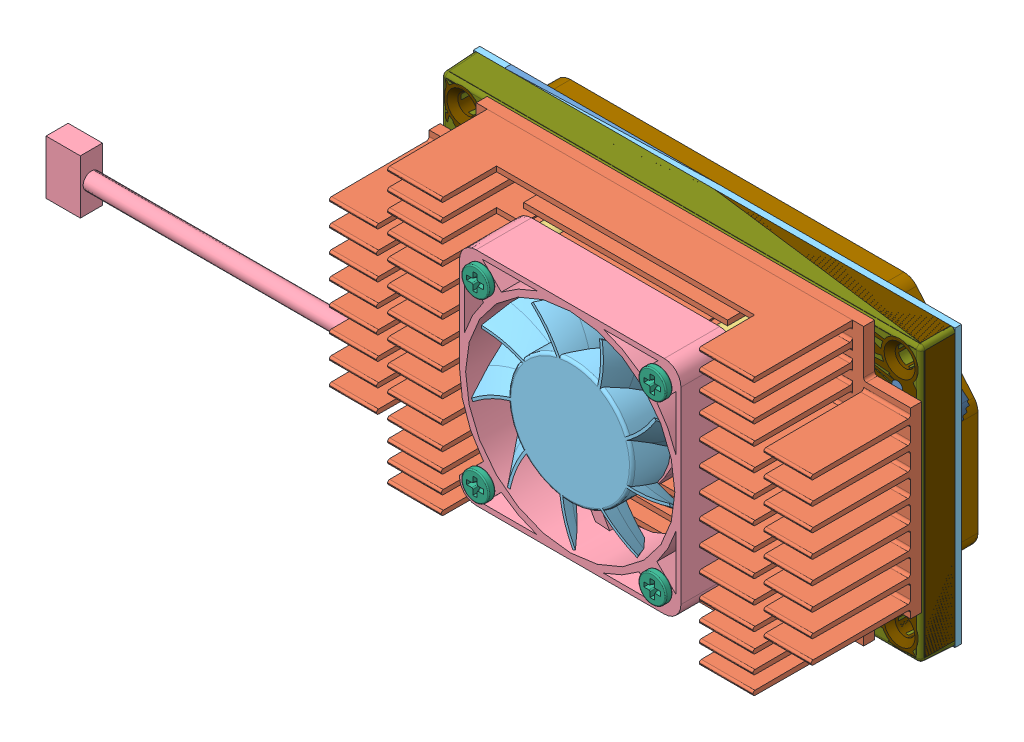
SolidWorks assembly JETSON-NEW_ASM, configuration Default. Lengths in mm. (continued)
Components (placement in the parent): (continued)
- 244-82180-1000-A01-07-31-15_ASM-1: 244-82180-1000-A01-07-31-15_ASM [Default] at origin size (87 50 8.3) (continued)
  - 195-2469-000_1-1: 195-2469-000_1 [Default] at (57.403 38.754 0) x (0 -1 0) z (0 0 -1) size (0.69 0.32 0.31)
  - 195-1636-000_1-61: 195-1636-000_1 [Default] at (57.19 37.076 0) x (-1 0 0) z (0 0 -1) size (0.69 0.32 0.31)
  - 195-1636-000_1-62: 195-1636-000_1 [Default] at (56.433 18.954 0) x (0 -1 0) z (0 0 -1) size (0.69 0.32 0.31)
  - 195-1636-000_1-63: 195-1636-000_1 [Default] at (56.153 17.514 0) x (1 0 0) z (0 0 -1) size (0.69 0.32 0.31)
  - 195-2006-000_1-13: 195-2006-000_1 [Default] at (56.153 18.064 0) x (1 0 0) z (0 0 -1) size (0.69 0.32 0.31)
  - 195-1636-000_1-64: 195-1636-000_1 [Default] at (56.153 16.294 0) x (-1 0 0) z (0 0 -1) size (0.69 0.32 0.31)
  - 195-2005-000_1-20: 195-2005-000_1 [Default] at (55.41 37.136 0) x (-1 0 0) z (0 0 -1) size (0.69 0.32 0.31)
  - 195-2005-000_1-21: 195-2005-000_1 [Default] at (54.515 37.047 0) x (1 0 0) z (0 0 -1) size (0.69 0.32 0.31)
  - 195-2004-000_1-2: 195-2004-000_1 [Default] at (54.515 36.527 0) x (1 0 0) z (0 0 -1) size (0.69 0.32 0.31)
  - 195-2004-000_1-3: 195-2004-000_1 [Default] at (54.515 36.007 0) x (1 0 0) z (0 0 -1) size (0.69 0.32 0.31)
  - 195-1636-000_1-65: 195-1636-000_1 [Default] at (56.3 37.076 0) x (1 0 0) z (0 0 -1) size (0.69 0.32 0.31)
  - 195-1636-000_1-66: 195-1636-000_1 [Default] at (69.95 41.15 0) x (-1 0 0) z (0 0 -1) size (0.69 0.32 0.31)
  - 039-0165-000_1-112: 039-0165-000_1 [Default] at (55.853 18.829 0) x (0 1 0) z (0 0 -1) size (0.69 0.32 0.34)
  - 195-2005-000_1-22: 195-2005-000_1 [Default] at (55.328 18.829 0) x (0 -1 0) z (0 0 -1) size (0.69 0.32 0.31)
  - 195-2173-000_1-1: 195-2173-000_1 [Default] at (55.063 17.794 0) x (-1 0 0) z (0 0 -1) size (0.69 0.32 0.31)
  - 195-2173-000_1-2: 195-2173-000_1 [Default] at (55.083 17.234 0) x (1 0 0) z (0 0 -1) size (0.69 0.32 0.31)
  - 039-0165-000_1-113: 039-0165-000_1 [Default] at (60.953 36.318 0) x (0 -1 0) z (0 0 -1) size (0.69 0.32 0.34)
  - 039-0165-000_1-114: 039-0165-000_1 [Default] at (59.253 34.954 0) x (1 0 0) z (0 0 -1) size (0.69 0.32 0.34)
  - 195-1636-000_1-67: 195-1636-000_1 [Default] at (59.32 33.596 0) x (0 1 0) z (0 0 -1) size (0.69 0.32 0.31)
  - 195-1636-000_1-68: 195-1636-000_1 [Default] at (59.85 33.596 0) x (0 1 0) z (0 0 -1) size (0.69 0.32 0.31)
  - 195-1636-000_1-69: 195-1636-000_1 [Default] at (61.26 31.736 0) x (-1 0 0) z (0 0 -1) size (0.69 0.32 0.31)
  - 195-1636-000_1-70: 195-1636-000_1 [Default] at (61.26 31.206 0) x (-1 0 0) z (0 0 -1) size (0.69 0.32 0.31)
  - 195-1636-000_1-71: 195-1636-000_1 [Default] at (58.65 38.25 0) x (0 1 0) z (0 0 -1) size (0.69 0.32 0.31)
  - 195-1636-000_1-72: 195-1636-000_1 [Default] at (58.103 37.754 0) x (0 -1 0) z (0 0 -1) size (0.69 0.32 0.31)
  - 039-0165-000_1-115: 039-0165-000_1 [Default] at (57.953 38.754 0) x (0 -1 0) z (0 0 -1) size (0.69 0.32 0.34)
  - 039-0165-000_1-116: 039-0165-000_1 [Default] at (58.08 36.986 0) x (1 0 0) z (0 0 -1) size (0.69 0.32 0.34)
  - 039-0165-000_1-117: 039-0165-000_1 [Default] at (58.06 36.446 0) x (1 0 0) z (0 0 -1) size (0.69 0.32 0.34)
  - 195-2005-000_1-23: 195-2005-000_1 [Default] at (61.853 39.434 0) x (1 0 0) z (0 0 -1) size (0.69 0.32 0.31)
  - 195-1636-000_1-73: 195-1636-000_1 [Default] at (62.063 38.899 0) x (1 0 0) z (0 0 -1) size (0.69 0.32 0.31)
  - 195-2117-000_1-9: 195-2117-000_1 [Default] at (62.2 37.35 0) x (1 0 0) z (0 0 -1) size (0.69 0.32 0.31)
  - 195-2350-000_1-1: 195-2350-000_1 [Default] at (62.2 35.7 0) x (1 0 0) z (0 0 -1) size (0.69 0.32 0.31)
  - 195-1636-000_1-74: 195-1636-000_1 [Default] at (61.31 33.856 0) x (1 0 0) z (0 0 -1) size (0.69 0.32 0.31)
  - 195-1636-000_1-75: 195-1636-000_1 [Default] at (61.31 33.326 0) x (1 0 0) z (0 0 -1) size (0.69 0.32 0.31)
  - 035-0122-000_1-15: 035-0122-000_1 [Default] at (61.585 32.427 1.164) x (-1 0 0) z (0 0 1) size (0.69 0.32 0.34)
  - 195-1636-000_1-76: 195-1636-000_1 [Default] at (61.31 32.796 0) x (1 0 0) z (0 0 -1) size (0.69 0.32 0.31)
  - 195-2171-000_1-3: 195-2171-000_1 [Default] at (61.98 31.446 0) x (0 1 0) z (0 0 -1) size (0.69 0.32 0.31)
  - 195-2171-000_1-4: 195-2171-000_1 [Default] at (62.7 31.736 0) x (-1 0 0) z (0 0 -1) size (0.69 0.32 0.31)
  - 195-2171-000_1-5: 195-2171-000_1 [Default] at (62.7 31.206 0) x (-1 0 0) z (0 0 -1) size (0.69 0.32 0.31)
  - 195-2006-000_1-14: 195-2006-000_1 [Default] at (61.35 17 0) x (-1 0 0) z (0 0 -1) size (0.69 0.32 0.31)
  - 195-2006-000_1-15: 195-2006-000_1 [Default] at (67.003 18.404 0) x (1 0 0) z (0 0 -1) size (0.69 0.32 0.31)
  - 195-1636-000_1-77: 195-1636-000_1 [Default] at (63.447 36.441 0) x (1 0 0) z (0 0 -1) size (0.69 0.32 0.31)
  - 195-2006-000_1-16: 195-2006-000_1 [Default] at (60.735 35.528 0) x (1 0 0) z (0 0 -1) size (0.69 0.32 0.31)
  - 195-2005-000_1-24: 195-2005-000_1 [Default] at (70.6 26.95 0) x (0 1 0) z (0 0 -1) size (0.69 0.32 0.31)
  - 195-1636-000_1-78: 195-1636-000_1 [Default] at (69 26.8 0) x (1 0 0) z (0 0 -1) size (0.69 0.32 0.31)
  - 195-2005-000_1-25: 195-2005-000_1 [Default] at (68.818 25.999 0) x (0 -1 0) z (0 0 -1) size (0.69 0.32 0.31)
  - 195-2173-000_1-3: 195-2173-000_1 [Default] at (68.073 25.764 0) x (-1 0 0) z (0 0 -1) size (0.69 0.32 0.31)
  - 195-1636-000_1-79: 195-1636-000_1 [Default] at (68.053 24.804 0) x (0 1 0) z (0 0 -1) size (0.69 0.32 0.31)
  - 195-2006-000_1-17: 195-2006-000_1 [Default] at (69.153 24.484 0) x (0 -1 0) z (0 0 -1) size (0.69 0.32 0.31)
  - 195-1636-000_1-80: 195-1636-000_1 [Default] at (68.913 25.224 0) x (1 0 0) z (0 0 -1) size (0.69 0.32 0.31)
  - 195-1636-000_1-81: 195-1636-000_1 [Default] at (68.603 24.484 0) x (0 -1 0) z (0 0 -1) size (0.69 0.32 0.31)
  - 035-0135-000_1-3: 035-0135-000_1 [Default] at (69.153 19.404 0) x (0 -1 0) z (0 0 -1) size (0.69 0.32 0.34)
  - 195-2274-000_1-1: 195-2274-000_1 [Default] at (68.553 19.404 0) x (0 -1 0) z (0 0 -1) size (0.69 0.32 0.31)
  - 039-0219-000_1-1: 039-0219-000_1 [Default] at (67.753 18.304 0) x (0 -1 0) z (0 0 -1) size (0.69 0.32 0.34)
  - 035-0135-000_1-4: 035-0135-000_1 [Default] at (68.653 18.604 0) x (1 0 0) z (0 0 -1) size (0.69 0.32 0.34)
  - 195-2173-000_1-4: 195-2173-000_1 [Default] at (67.133 25.764 0) x (1 0 0) z (0 0 -1) size (0.69 0.32 0.31)
  - 195-2004-000_1-4: 195-2004-000_1 [Default] at (18.25 37.45 0) x (0 1 0) z (0 0 -1) size (0.69 0.32 0.31)
  - 195-2004-000_1-5: 195-2004-000_1 [Default] at (18.8 37.45 0) x (0 1 0) z (0 0 -1) size (0.69 0.32 0.31)
  - 195-1636-000_1-82: 195-1636-000_1 [Default] at (41.75 9 1.164) x (0 -1 0) z (0 0 1) size (0.69 0.32 0.31)
  - 195-2459-000_1-1: 195-2459-000_1 [Default] at (70.675 24.972 0) x (0 1 0) z (0 0 -1) size (0.69 0.32 0.31)
  - 195-1636-000_1-83: 195-1636-000_1 [Default] at (70.053 24.254 0) x (1 0 0) z (0 0 -1) size (0.69 0.32 0.31)
  - 039-0165-000_1-118: 039-0165-000_1 [Default] at (69.903 24.854 0) x (1 0 0) z (0 0 -1) size (0.69 0.32 0.34)
  - 195-1636-000_1-84: 195-1636-000_1 [Default] at (70.753 20.604 0) x (0 -1 0) z (0 0 -1) size (0.69 0.32 0.31)
  - 035-0135-000_1-5: 035-0135-000_1 [Default] at (70.553 19.284 0) x (1 0 0) z (0 0 -1) size (0.69 0.32 0.34)
  - 195-2172-000_1-4: 195-2172-000_1 [Default] at (70.553 19.804 0) x (1 0 0) z (0 0 -1) size (0.69 0.32 0.31)
  - 035-0135-000_1-6: 035-0135-000_1 [Default] at (69.753 19.404 0) x (0 -1 0) z (0 0 -1) size (0.69 0.32 0.34)
  - 195-2172-000_1-5: 195-2172-000_1 [Default] at (70.253 18.004 0) x (1 0 0) z (0 0 -1) size (0.69 0.32 0.31)
  - 195-1636-000_1-85: 195-1636-000_1 [Default] at (70.253 18.604 0) x (1 0 0) z (0 0 -1) size (0.69 0.32 0.31)
  - 035-0135-000_1-7: 035-0135-000_1 [Default] at (71.25 18 0) x (1 0 0) z (0 0 -1) size (0.69 0.32 0.34)
  - 195-2002-000_1-6: 195-2002-000_1 [Default] at (68.9 33 0) x (0 1 0) z (0 0 -1) size (0.69 0.32 0.31)
  - 195-2002-000_1-7: 195-2002-000_1 [Default] at (73.4 30.6 0) x (1 0 0) z (0 0 -1) size (0.69 0.32 0.31)
  - 195-2319-000_1-1: 195-2319-000_1 [Default] at (70.953 23.922 0) x (-1 0 0) z (0 0 -1) size (0.69 0.32 0.31)
  - 039-0199-000_1-2: 039-0199-000_1 [Default] at (70.953 22.804 0) x (1 0 0) z (0 0 -1) size (0.69 0.32 0.36)
  - 195-2299-000_1-1: 195-2299-000_1 [Default] at (71.853 22.804 0) x (-1 0 0) z (0 0 -1) size (0.69 0.32 0.31)
  - 195-2289-000_1-1: 195-2289-000_1 [Default] at (70.953 23.404 0) x (1 0 0) z (0 0 -1) size (0.69 0.32 0.31)
  - 195-1636-000_1-86: 195-1636-000_1 [Default] at (71.853 23.404 0) x (1 0 0) z (0 0 -1) size (0.69 0.32 0.31)
  - 032-0335-000_1-1: 032-0335-000_1 [Default] at (71.553 20.804 0) x (-1 0 0) z (0 0 -1) size (0.69 0.32 0.34)
  - 195-2173-000_1-5: 195-2173-000_1 [Default] at (70.953 21.404 0) x (-1 0 0) z (0 0 -1) size (0.69 0.32 0.31)
  - 195-2061-000_1-1: 195-2061-000_1 [Default] at (71.853 21.404 0) x (-1 0 0) z (0 0 -1) size (0.69 0.32 0.31)
  - 195-2548-000_1-1: 195-2548-000_1 [Default] at (70.953 22.204 0) x (1 0 0) z (0 0 -1) size (0.69 0.32 0.31)
  - 039-0165-000_1-119: 039-0165-000_1 [Default] at (71.853 22.204 0) x (1 0 0) z (0 0 -1) size (0.69 0.32 0.34)
  - 195-1636-000_1-87: 195-1636-000_1 [Default] at (72.5 19.9 0) x (1 0 0) z (0 0 -1) size (0.69 0.32 0.31)
  - 195-2003-000_1-1: 195-2003-000_1 [Default] at (71.25 18.6 0) x (1 0 0) z (0 0 -1) size (0.69 0.32 0.31)
  - 036-0107-000_1-1: 036-0107-000_1 [Default] at (71.553 19.304 0) x (1 0 0) z (0 0 -1) size (0.69 0.32 0.31)
  - 195-1636-000_1-88: 195-1636-000_1 [Default] at (71.553 19.904 0) x (1 0 0) z (0 0 -1) size (0.69 0.32 0.31)
  - 195-1636-000_1-89: 195-1636-000_1 [Default] at (72.5 19.3 0) x (1 0 0) z (0 0 -1) size (0.69 0.32 0.31)
  - 195-2003-000_1-2: 195-2003-000_1 [Default] at (72.5 20.45 0) x (1 0 0) z (0 0 -1) size (0.69 0.32 0.31)
  - 195-2002-000_1-8: 195-2002-000_1 [Default] at (74.5 30.3 0) x (1 0 0) z (0 0 -1) size (0.69 0.32 0.31)
  - 195-2002-000_1-9: 195-2002-000_1 [Default] at (77.75 33.4 0) x (1 0 0) z (0 0 -1) size (0.69 0.32 0.31)
  - 195-1636-000_1-90: 195-1636-000_1 [Default] at (74.65 29.5 0) x (0 1 0) z (0 0 -1) size (0.69 0.32 0.31)
  - 195-2002-000_1-10: 195-2002-000_1 [Default] at (73.55 31.15 0) x (-1 0 0) z (0 0 -1) size (0.69 0.32 0.31)
  - 195-1636-000_1-91: 195-1636-000_1 [Default] at (74.55 37.6 0) x (0 -1 0) z (0 0 -1) size (0.69 0.32 0.31)
  - 035-0243-000_2-23: 035-0243-000_2 [Default] at (21.1 29.15 1.164) x (0 -1 0) z (0 0 1) size (0.69 0.32 0.34)
  - 035-0243-000_2-24: 035-0243-000_2 [Default] at (22.3 24.7 1.164) x (-1 0 0) z (0 0 1) size (0.69 0.32 0.34)
  - 195-2004-000_1-6: 195-2004-000_1 [Default] at (18.35 20.85 1.164) size (0.69 0.32 0.31)
  - 195-2004-000_1-7: 195-2004-000_1 [Default] at (18.35 21.4 1.164) size (0.69 0.32 0.31)
  - 195-2057-000_1-1: 195-2057-000_1 [Default] at (26.4 22.45 1.164) x (0 -1 0) z (0 0 1) size (0.69 0.32 0.31)
  - 195-2117-000_1-10: 195-2117-000_1 [Default] at (17.2 23.15 0) x (1 0 0) z (0 0 -1) size (0.69 0.32 0.31)
  - 195-2117-000_1-11: 195-2117-000_1 [Default] at (17.2 24.25 0) x (1 0 0) z (0 0 -1) size (0.69 0.32 0.31)
  - 195-2117-000_1-12: 195-2117-000_1 [Default] at (18.55 15.5 0) x (1 0 0) z (0 0 -1) size (0.69 0.32 0.31)
  - 195-2117-000_1-13: 195-2117-000_1 [Default] at (17.6 15.5 0) x (1 0 0) z (0 0 -1) size (0.69 0.32 0.31)
  - 195-2117-000_1-14: 195-2117-000_1 [Default] at (17.6 17.19 0) x (1 0 0) z (0 0 -1) size (0.69 0.32 0.31)
  - 195-1636-000_1-92: 195-1636-000_1 [Default] at (19.785 34.602 0) x (0 1 0) z (0 0 -1) size (0.69 0.32 0.31)
  - 195-1636-000_1-93: 195-1636-000_1 [Default] at (19.267 34.602 0) x (0 1 0) z (0 0 -1) size (0.69 0.32 0.31)
  - 195-1636-000_1-94: 195-1636-000_1 [Default] at (51.7 24.8 0) x (0 1 0) z (0 0 -1) size (0.69 0.32 0.31)
  - 035-0243-000_2-25: 035-0243-000_2 [Default] at (48.05 23.5 1.164) x (0 1 0) z (0 0 1) size (0.69 0.32 0.34)
  - 039-0165-000_1-120: 039-0165-000_1 [Default] at (41.543 22.374 0) x (0 -1 0) z (0 0 -1) size (0.69 0.32 0.34)
  - 039-0165-000_1-121: 039-0165-000_1 [Default] at (40.833 22.824 0) x (-1 0 0) z (0 0 -1) size (0.69 0.32 0.34)
  - 195-2007-000_1-1: 195-2007-000_1 [Default] at (18.65 12.6 0) x (0 -1 0) z (0 0 -1) size (0.69 0.32 0.31)
  - 195-1636-000_1-95: 195-1636-000_1 [Default] at (-0.85 36.75 1.164) x (-1 0 0) z (0 0 1) size (0.69 0.32 0.31)
  - 035-0243-000_2-26: 035-0243-000_2 [Default] at (-0.1 36.5 1.164) x (0 -1 0) z (0 0 1) size (0.69 0.32 0.34)
  - 035-0105-000_1-9: 035-0105-000_1 [Default] at (0.65 36.75 1.164) size (0.69 0.32 0.34)
  - 195-1636-000_1-96: 195-1636-000_1 [Default] at (-0.85 31.15 1.164) x (-1 0 0) z (0 0 1) size (0.69 0.32 0.31)
  - 035-0243-000_2-27: 035-0243-000_2 [Default] at (-0.1 30.9 1.164) x (0 -1 0) z (0 0 1) size (0.69 0.32 0.34)
  - 035-0105-000_1-10: 035-0105-000_1 [Default] at (0.65 31.15 1.164) size (0.69 0.32 0.34)
  - 035-0122-000_1-16: 035-0122-000_1 [Default] at (57.665 22.463 0) x (0 -1 0) z (0 0 -1) size (0.69 0.32 0.34)
  - 195-2566-000_1-1: 195-2566-000_1 [Default] at (31.05 10.1 1.164) x (0 -1 0) z (0 0 1) size (0.69 0.32 0.31)
  - 195-1636-000_1-97: 195-1636-000_1 [Default] at (64.54 30.986 0) x (-1 0 0) z (0 0 -1) size (0.69 0.32 0.31)
  - 195-1636-000_1-98: 195-1636-000_1 [Default] at (63.6 30.986 0) x (1 0 0) z (0 0 -1) size (0.69 0.32 0.31)
  - 195-1636-000_1-99: 195-1636-000_1 [Default] at (62.7 32.266 0) x (-1 0 0) z (0 0 -1) size (0.69 0.32 0.31)
  - 195-1636-000_1-100: 195-1636-000_1 [Default] at (61.26 32.266 0) x (-1 0 0) z (0 0 -1) size (0.69 0.32 0.31)
  - 036-0107-000_1-2: 036-0107-000_1 [Default] at (64.28 32.246 0) x (1 0 0) z (0 0 -1) size (0.69 0.32 0.31)
  - 195-2566-000_1-2: 195-2566-000_1 [Default] at (45.8 23.3 1.164) x (0 1 0) z (0 0 1) size (0.69 0.32 0.31)
  - 195-2319-000_1-2: 195-2319-000_1 [Default] at (56.55 19.856 0) x (0 -1 0) z (0 0 -1) size (0.69 0.32 0.31)
  - 195-2299-000_1-2: 195-2299-000_1 [Default] at (58.55 21.116 0) x (-1 0 0) z (0 0 -1) size (0.69 0.32 0.31)
  - 195-2289-000_1-2: 195-2289-000_1 [Default] at (57.09 19.856 0) x (0 1 0) z (0 0 -1) size (0.69 0.32 0.31)
  - 195-1636-000_1-101: 195-1636-000_1 [Default] at (58.55 21.656 0) x (1 0 0) z (0 0 -1) size (0.69 0.32 0.31)
  - 032-0335-000_1-2: 032-0335-000_1 [Default] at (58.55 20.576 0) x (-1 0 0) z (0 0 -1) size (0.69 0.32 0.34)
  - 039-0199-000_1-3: 039-0199-000_1 [Default] at (57.63 19.856 0) x (0 1 0) z (0 0 -1) size (0.69 0.32 0.36)
  - 039-0204-000_1-1: 039-0204-000_1 [Default] at (71.45 25.1 0) x (-1 0 0) z (0 0 -1) size (0.69 0.32 0.34)
  - 039-0204-000_1-2: 039-0204-000_1 [Default] at (58.17 19.856 0) x (0 1 0) z (0 0 -1) size (0.69 0.32 0.34)
  - 195-1636-000_1-102: 195-1636-000_1 [Default] at (71.453 24.573 0) x (1 0 0) z (0 0 -1) size (0.69 0.32 0.31)
  - 195-1636-000_1-103: 195-1636-000_1 [Default] at (58.74 19.856 0) x (0 -1 0) z (0 0 -1) size (0.69 0.32 0.31)
  - 101-0142-000_2-1: 101-0142-000_2 [Default] at (6.063 36.964 1.164) x (0 1 0) z (0 0 1) size (1.4 1.1 0.4)
  - 101-0142-000_2-2: 101-0142-000_2 [Default] at (5.31 31.454 1.164) x (0 1 0) z (0 0 1) size (1.4 1.1 0.4)
  - 085-0203-000_1-1: 085-0203-000_1 [Default] at (13.653 29.754 1.164) size (1.75 1.35 0.4)
  - 131-0802-000_2-1: 131-0802-000_2 [Default] at (18.469 28.798 1.164) x (0 -1 0) z (0 0 1) size (2.53 1.61 1.01)
  - 085-0180-000_1-1: 085-0180-000_1 [Default] at (23.25 23 1.164) x (-1 0 0) z (0 0 1) size (2.9 2.5 0.56)
  - 305-0057-000_1-1: 305-0057-000_1 [Default] at (41.153 40.254 0) x (1 0 0) z (0 0 -1) size (2 2.69 1.1)
  - 115-0057-000_1-1: 115-0057-000_1 [Default] at (1.1 13.65 0) x (-1 0 0) z (0 0 -1) size (2 2.88 1.1)
  - 115-1572-000_1-1: 115-1572-000_1 [Default] at (65.88 15.256 0) x (0 -1 0) z (0 0 -1) size (2 2.88 1.1)
  - 315-0217-000_1-1: 315-0217-000_1 [Default] at (41.273 36.727 0) x (1 0 0) z (0 0 -1) size (2 2.88 1.1)
  - 032-0627-000_1-1: 032-0627-000_1 [Default] at (1.38 7.93 1.164) x (-1 0 0) z (0 0 1) size (4.22 2.82 1.2)
  - 032-0627-000_1-2: 032-0627-000_1 [Default] at (68.106 40.15 1.164) x (0 -1 0) z (0 0 1) size (4.22 2.82 1.2)
  - 032-0627-000_1-3: 032-0627-000_1 [Default] at (72.09 40.46 1.164) size (4.22 2.82 1.2)
  - 032-0627-000_1-4: 032-0627-000_1 [Default] at (1.38 11.27 1.164) x (-1 0 0) z (0 0 1) size (4.22 2.82 1.2)
  - 032-0636-000_1-1: 032-0636-000_1 [Default] at (47.778 13.049 0) x (1 0 0) z (0 0 -1) size (4.22 2.82 1.5)
  - 032-0471-000_2-1: 032-0471-000_2 [Default] at (47.78 16.326 0) x (1 0 0) z (0 0 -1) size (4.22 2.82 1.2)
  - 032-0636-000_1-2: 032-0636-000_1 [Default] at (54.36 22.056 0) x (0 -1 0) z (0 0 -1) size (4.22 2.82 1.5)
  - 032-0471-000_2-2: 032-0471-000_2 [Default] at (36.91 17.143 0) x (-1 0 0) z (0 0 -1) size (4.22 2.82 1.2)
  - 032-0471-000_2-3: 032-0471-000_2 [Default] at (49.67 19.576 0) x (1 0 0) z (0 0 -1) size (4.22 2.82 1.2)
  - 130-0646-000_1-1: 130-0646-000_1 [Default] at (57.753 23.554 1.164) x (-1 0 0) z (0 0 1) size (8.4 6.6 1.8)
  - 130-0646-000_1-2: 130-0646-000_1 [Default] at (57.753 16.304 1.164) x (-1 0 0) z (0 0 1) size (8.4 6.6 1.8)
  - 130-0562-000_2-1: 130-0562-000_2 [Default] at (56.978 30.96 1.164) x (0 -1 0) z (0 0 1) size (2.8 2.25 1.22)
  - 130-0562-000_2-2: 130-0562-000_2 [Default] at (53.858 37.854 1.164) x (0 1 0) z (0 0 1) size (2.8 2.25 1.22)
  - 130-0562-000_2-3: 130-0562-000_2 [Default] at (53.848 33.894 1.164) x (0 -1 0) z (0 0 1) size (2.8 2.25 1.22)
  - 130-0562-000_2-4: 130-0562-000_2 [Default] at (59.478 30.965 1.164) x (0 -1 0) z (0 0 1) size (2.8 2.25 1.22)
  - 130-0562-000_2-5: 130-0562-000_2 [Default] at (63.578 33.764 1.164) x (0 -1 0) z (0 0 1) size (2.8 2.25 1.22)
  - 300-0252-000_1-1: 300-0252-000_1 [Default] at (63.7 17.8 1.164) x (0 -1 0) z (0 0 1) size (3.81 3.5 0.81)
  - 300-0252-000_1-2: 300-0252-000_1 [Default] at (63.7 22.25 1.164) x (0 1 0) z (0 0 1) size (3.81 3.5 0.81)
  - 300-0252-000_1-3: 300-0252-000_1 [Default] at (63.7 13.55 1.164) x (0 1 0) z (0 0 1) size (3.81 3.5 0.81)
  - 300-0252-000_1-4: 300-0252-000_1 [Default] at (63.7 26.5 1.164) x (0 -1 0) z (0 0 1) size (3.81 3.5 0.81)
  - 300-0284-000_1-1: 300-0284-000_1 [Default] at (67.9 22.7 1.164) size (3.81 3.5 0.81)
  - 300-0284-000_1-2: 300-0284-000_1 [Default] at (67.9 15.45 1.164) size (3.81 3.5 0.81)
  - 039-0208-000_1-1: 039-0208-000_1 [Default] at (4.01 9.61 1.164) x (0 1 0) z (0 0 1) size (1.2 0.5 0.55)
  - 039-0208-000_1-2: 039-0208-000_1 [Default] at (73.36 37.97 1.164) size (1.2 0.5 0.55)
  - 032-0204-000_2-1: 032-0204-000_2 [Default] at (69.95 26.3 0) x (0 1 0) z (0 0 -1) size (1.2 0.5 0.55)
  - 195-0486-000_1-1: 195-0486-000_1 [Default] at (9.75 33.6 0) x (-1 0 0) z (0 0 -1) size (1.2 0.5 0.4)
  - 195-0324-000_1-1: 195-0324-000_1 [Default] at (10.2 30.95 0) x (0 -1 0) z (0 0 -1) size (1.2 0.5 0.4)
  - 195-0235-000_1-1: 195-0235-000_1 [Default] at (9.4 32.45 0) x (0 -1 0) z (0 0 -1) size (1.2 0.5 0.4)
  - 036-0014-000_1-1: 036-0014-000_1 [Default] at (6.25 30.3 0) x (1 0 0) z (0 0 -1) size (1.2 0.5 0.6)
  - 036-0014-000_1-2: 036-0014-000_1 [Default] at (9.4 30.95 0) x (0 -1 0) z (0 0 -1) size (1.2 0.5 0.6)
  - 195-1691-000_1-1: 195-1691-000_1 [Default] at (44.62 11.876 0) x (0 1 0) z (0 0 -1) size (1.2 0.5 0.4)
  - 195-1691-000_1-2: 195-1691-000_1 [Default] at (43.89 11.876 0) x (0 1 0) z (0 0 -1) size (1.2 0.5 0.4)
  - 195-0415-000_1-1: 195-0415-000_1 [Default] at (74.79 39.5 1.164) x (0 1 0) z (0 0 1) size (1.2 0.5 0.4)
  - 035-0017-000_1-1: 035-0017-000_1 [Default] at (76.18 34.056 1.164) x (0 -1 0) z (0 0 1) size (1.2 0.5 0.6)
  - 195-0210-000_1-1: 195-0210-000_1 [Default] at (77.99 35.336 1.164) size (1.2 0.5 0.4)
  - 195-0475-000_1-1: 195-0475-000_1 [Default] at (77.98 34.596 1.164) x (-1 0 0) z (0 0 1) size (1.2 0.5 0.4)
  - 036-0141-000_1-1: 036-0141-000_1 [Default] at (76.93 34.056 1.164) x (0 -1 0) z (0 0 1) size (1.2 0.5 0.61)
  - 195-0070-000_1-1: 195-0070-000_1 [Default] at (76.53 35.156 1.164) size (1.2 0.5 0.4)
  - 035-0212-000_1-1: 035-0212-000_1 [Default] at (77.69 32.384 1.164) x (0 1 0) z (0 0 1) size (1.2 0.5 0.55)
  - 195-0005-000_1-1: 195-0005-000_1 [Default] at (76.97 32.384 1.164) x (0 1 0) z (0 0 1) size (1.2 0.5 0.4)
  - 195-0140-000_1-1: 195-0140-000_1 [Default] at (75.74 32.814 1.164) x (-1 0 0) z (0 0 1) size (1.2 0.5 0.4)
  - 195-0342-000_1-1: 195-0342-000_1 [Default] at (75.776 31.96 1.164) size (1.2 0.5 0.4)
  - 195-0405-000_1-1: 195-0405-000_1 [Default] at (2.04 14.56 1.164) x (-1 0 0) z (0 0 1) size (1.2 0.5 0.4)
  - 035-0212-000_1-2: 035-0212-000_1 [Default] at (8.776 12.06 1.164) x (0 -1 0) z (0 0 1) size (1.2 0.5 0.55)
  - 195-0487-000_1-1: 195-0487-000_1 [Default] at (0.83 14.77 1.164) x (0 1 0) z (0 0 1) size (1.2 0.5 0.4)
  - 195-0240-000_1-1: 195-0240-000_1 [Default] at (-0.384 15.76 1.164) x (0 -1 0) z (0 0 1) size (1.2 0.5 0.4)
  - 036-0141-000_1-2: 036-0141-000_1 [Default] at (9.126 10.96 1.164) x (-1 0 0) z (0 0 1) size (1.2 0.5 0.61)
  - 195-0404-000_1-1: 195-0404-000_1 [Default] at (9.526 12.06 1.164) x (0 -1 0) z (0 0 1) size (1.2 0.5 0.4)
  - 035-0212-000_1-3: 035-0212-000_1 [Default] at (10.24 9.756 1.164) x (0 -1 0) z (0 0 1) size (1.2 0.5 0.55)
  - 195-0342-000_1-2: 195-0342-000_1 [Default] at (11.404 10.18 1.164) x (-1 0 0) z (0 0 1) size (1.2 0.5 0.4)
  - 195-0005-000_1-2: 195-0005-000_1 [Default] at (9.53 9.756 1.164) x (0 -1 0) z (0 0 1) size (1.2 0.5 0.4)
  - 195-0250-000_1-1: 195-0250-000_1 [Default] at (8.664 9.78 1.164) x (0 1 0) z (0 0 1) size (1.2 0.5 0.4)
  - 195-0485-000_1-1: 195-0485-000_1 [Default] at (5.7 11.85 0) x (-1 0 0) z (0 0 -1) size (1.2 0.5 0.4)
  - 195-0485-000_1-2: 195-0485-000_1 [Default] at (5.7 12.6 0) x (-1 0 0) z (0 0 -1) size (1.2 0.5 0.4)
  - 039-0023-000_1-1: 039-0023-000_1 [Default] at (36.871 31.058 0) x (-1 0 0) z (0 0 -1) size (1.2 0.5 0.6)
  - 195-0031-000_1-1: 195-0031-000_1 [Default] at (35.801 30.61 0) x (0 1 0) z (0 0 -1) size (1.2 0.5 0.4)
  - 195-2655-000_1-1: 195-2655-000_1 [Default] at (36.871 30.308 0) x (-1 0 0) z (0 0 -1) size (1.2 0.5 0.4)
  - 195-0437-000_1-1: 195-0437-000_1 [Default] at (36.479 24.219 0) x (0 -1 0) z (0 0 -1) size (1.2 0.5 0.4)
  - 195-0292-000_1-1: 195-0292-000_1 [Default] at (35.427 24.921 0) x (-1 0 0) z (0 0 -1) size (1.2 0.5 0.4)
  - 039-0008-000_1-1: 039-0008-000_1 [Default] at (39.63 37.104 0) x (0 -1 0) z (0 0 -1) size (1.2 0.5 0.6)
  - 039-0008-000_1-2: 039-0008-000_1 [Default] at (41.103 34.754 0) x (1 0 0) z (0 0 -1) size (1.2 0.5 0.6)
  - 195-0484-000_1-1: 195-0484-000_1 [Default] at (46.963 29.024 0) x (1 0 0) z (0 0 -1) size (1.2 0.5 0.4)
  - 195-0596-000_1-1: 195-0596-000_1 [Default] at (46.963 28.214 0) x (1 0 0) z (0 0 -1) size (1.2 0.5 0.4)
  - 195-0002-000_1-1: 195-0002-000_1 [Default] at (52.188 28.414 0) x (-1 0 0) z (0 0 -1) size (1.2 0.5 0.4)
  - 036-0012-000_1-1: 036-0012-000_1 [Default] at (51.053 28.084 0) x (0 -1 0) z (0 0 -1) size (1.2 0.5 0.6)
  - 195-0486-000_1-2: 195-0486-000_1 [Default] at (69.45 10.95 1.164) size (1.2 0.5 0.4)
  - 039-0008-000_1-3: 039-0008-000_1 [Default] at (11.5 19.1 0) x (0 -1 0) z (0 0 -1) size (1.2 0.5 0.6)
  - 195-2655-000_1-2: 195-2655-000_1 [Default] at (19.934 31.265 0) x (0 -1 0) z (0 0 -1) size (1.2 0.5 0.4)
  - 039-0008-000_1-4: 039-0008-000_1 [Default] at (21.486 32.341 0) x (-1 0 0) z (0 0 -1) size (1.2 0.5 0.6)
  - 195-2655-000_1-3: 195-2655-000_1 [Default] at (20.641 31.27 0) x (0 -1 0) z (0 0 -1) size (1.2 0.5 0.4)
  - 039-0136-000_1-1: 039-0136-000_1 [Default] at (10.606 31.182 1.164) x (-0.707107 -0.707107 0) z (0 0 1) size (1.2 0.5 0.61)
  - 039-0136-000_1-2: 039-0136-000_1 [Default] at (12.104 29.849 1.164) x (0 1 0) z (0 0 1) size (1.2 0.5 0.61)
  - 039-0136-000_1-3: 039-0136-000_1 [Default] at (11.729 28.799 1.164) x (-1 0 0) z (0 0 1) size (1.2 0.5 0.61)
  - 039-0136-000_1-4: 039-0136-000_1 [Default] at (14.693 27.88 1.164) x (-1 0 0) z (0 0 1) size (1.2 0.5 0.61)
  - 039-0136-000_1-5: 039-0136-000_1 [Default] at (12.197 36.147 1.164) x (-1 0 0) z (0 0 1) size (1.2 0.5 0.61)
  - 039-0008-000_1-5: 039-0008-000_1 [Default] at (13.012 34.245 0) x (0 1 0) z (0 0 -1) size (1.2 0.5 0.6)
  - 195-2655-000_1-4: 195-2655-000_1 [Default] at (13.563 33.192 0) x (1 0 0) z (0 0 -1) size (1.2 0.5 0.4)
  - 039-0136-000_1-6: 039-0136-000_1 [Default] at (13.208 27.925 1.164) x (-1 0 0) z (0 0 1) size (1.2 0.5 0.61)
  - 195-2655-000_1-5: 195-2655-000_1 [Default] at (18.836 32.716 0) x (0 -1 0) z (0 0 -1) size (1.2 0.5 0.4)
  - 032-0153-000_2-1: 032-0153-000_2 [Default] at (17.436 32.716 0) x (0 1 0) z (0 0 -1) size (1.2 0.5 0.6)
  - 039-0008-000_1-6: 039-0008-000_1 [Default] at (14.75 39.45 0) x (-1 0 0) z (0 0 -1) size (1.2 0.5 0.6)
  - 195-2655-000_1-6: 195-2655-000_1 [Default] at (15.15 38.25 0) x (0 1 0) z (0 0 -1) size (1.2 0.5 0.4)
  - 039-0008-000_1-7: 039-0008-000_1 [Default] at (15.15 42.05 0) x (0 1 0) z (0 0 -1) size (1.2 0.5 0.6)
  - 039-0136-000_1-7: 039-0136-000_1 [Default] at (16.088 35.815 0) x (0 1 0) z (0 0 -1) size (1.2 0.5 0.61)
  - 039-0136-000_1-8: 039-0136-000_1 [Default] at (16.036 33.333 0) x (0 1 0) z (0 0 -1) size (1.2 0.5 0.61)
  - 039-0008-000_1-8: 039-0008-000_1 [Default] at (17.786 33.809 0) x (1 0 0) z (0 0 -1) size (1.2 0.5 0.6)
  - 039-0011-000_1-1: 039-0011-000_1 [Default] at (16.736 32.933 0) x (0 1 0) z (0 0 -1) size (1.2 0.5 0.6)
  - 039-0136-000_1-9: 039-0136-000_1 [Default] at (15.842 29.849 1.164) x (0 -1 0) z (0 0 1) size (1.2 0.5 0.61)
  - 032-0153-000_2-2: 032-0153-000_2 [Default] at (17.068 29.641 1.164) x (0 -1 0) z (0 0 1) size (1.2 0.5 0.6)
  - 195-2655-000_1-7: 195-2655-000_1 [Default] at (27.6 19.65 0) x (0 -1 0) z (0 0 -1) size (1.2 0.5 0.4)
  - 039-0008-000_1-9: 039-0008-000_1 [Default] at (26.268 14.214 0) x (0 1 0) z (0 0 -1) size (1.2 0.5 0.6)
  - 195-2655-000_1-8: 195-2655-000_1 [Default] at (24.438 17.784 0) x (1 0 0) z (0 0 -1) size (1.2 0.5 0.4)
  - 039-0008-000_1-10: 039-0008-000_1 [Default] at (25.473 16.544 0) x (0 -1 0) z (0 0 -1) size (1.2 0.5 0.6)
  - 039-0008-000_1-11: 039-0008-000_1 [Default] at (25.032 13.913 0) x (1 0 0) z (0 0 -1) size (1.2 0.5 0.6)
  - 039-0008-000_1-12: 039-0008-000_1 [Default] at (23.442 16.554 0) x (0 -1 0) z (0 0 -1) size (1.2 0.5 0.6)
  - 039-0008-000_1-13: 039-0008-000_1 [Default] at (33.563 14.704 0) x (0 1 0) z (0 0 -1) size (1.2 0.5 0.6)
  - 039-0008-000_1-14: 039-0008-000_1 [Default] at (39.241 18.025 0) x (1 0 0) z (0 0 -1) size (1.2 0.5 0.6)
  - 039-0008-000_1-15: 039-0008-000_1 [Default] at (37.923 13.224 0) x (0 -1 0) z (0 0 -1) size (1.2 0.5 0.6)
  - 039-0008-000_1-16: 039-0008-000_1 [Default] at (36.533 21.324 0) x (0 -1 0) z (0 0 -1) size (1.2 0.5 0.6)
  - 039-0008-000_1-17: 039-0008-000_1 [Default] at (36.883 19.644 0) x (0 -1 0) z (0 0 -1) size (1.2 0.5 0.6)
  - 039-0008-000_1-18: 039-0008-000_1 [Default] at (36.423 14.689 0) x (0 -1 0) z (0 0 -1) size (1.2 0.5 0.6)
  - 039-0008-000_1-19: 039-0008-000_1 [Default] at (34.543 20.894 0) x (-1 0 0) z (0 0 -1) size (1.2 0.5 0.6)
  - 039-0008-000_1-20: 039-0008-000_1 [Default] at (43.6 19.15 0) x (0 1 0) z (0 0 -1) size (1.2 0.5 0.6)
  - 039-0008-000_1-21: 039-0008-000_1 [Default] at (34.282 15.951 0) x (0 1 0) z (0 0 -1) size (1.2 0.5 0.6)
  - 039-0008-000_1-22: 039-0008-000_1 [Default] at (39.653 19.654 0) x (0 -1 0) z (0 0 -1) size (1.2 0.5 0.6)
  - 039-0008-000_1-23: 039-0008-000_1 [Default] at (40.423 13.214 0) x (0 -1 0) z (0 0 -1) size (1.2 0.5 0.6)
  - 195-2655-000_1-9: 195-2655-000_1 [Default] at (39.163 11.574 0) x (0 1 0) z (0 0 -1) size (1.2 0.5 0.4)
  - 035-0012-000_1-1: 035-0012-000_1 [Default] at (66.85 13.326 0) x (0 -1 0) z (0 0 -1) size (1.2 0.5 0.6)
  - 195-0315-000_1-1: 195-0315-000_1 [Default] at (66.1 13.326 0) x (0 -1 0) z (0 0 -1) size (1.2 0.5 0.4)
  - 195-0005-000_1-3: 195-0005-000_1 [Default] at (65.35 13.326 0) x (0 -1 0) z (0 0 -1) size (1.2 0.5 0.4)
  - 195-0200-000_1-1: 195-0200-000_1 [Default] at (69.4 15.1 0) x (0 1 0) z (0 0 -1) size (1.2 0.5 0.4)
  - 039-0008-000_1-24: 039-0008-000_1 [Default] at (43.95 20.2 0) x (1 0 0) z (0 0 -1) size (1.2 0.5 0.6)
  - 195-2655-000_1-10: 195-2655-000_1 [Default] at (65.838 16.894 0) x (1 0 0) z (0 0 -1) size (1.2 0.5 0.4)
  - 039-0008-000_1-25: 039-0008-000_1 [Default] at (46.11 16.806 1.164) x (0 -1 0) z (0 0 1) size (1.2 0.5 0.6)
  - 039-0008-000_1-26: 039-0008-000_1 [Default] at (44.65 19.1 0) x (0 1 0) z (0 0 -1) size (1.2 0.5 0.6)
  - 195-0485-000_1-3: 195-0485-000_1 [Default] at (50.55 26.4 0) x (0 1 0) z (0 0 -1) size (1.2 0.5 0.4)
  - 195-0485-000_1-4: 195-0485-000_1 [Default] at (49.85 26.4 0) x (0 1 0) z (0 0 -1) size (1.2 0.5 0.4)
  - 195-0005-000_1-4: 195-0005-000_1 [Default] at (68.7 15.1 0) x (0 1 0) z (0 0 -1) size (1.2 0.5 0.4)
  - 039-0008-000_1-27: 039-0008-000_1 [Default] at (45.55 21.7 1.164) x (-1 0 0) z (0 0 1) size (1.2 0.5 0.6)
  - 039-0008-000_1-28: 039-0008-000_1 [Default] at (45.36 16.806 1.164) x (0 -1 0) z (0 0 1) size (1.2 0.5 0.6)
  - 036-0014-000_1-3: 036-0014-000_1 [Default] at (59.75 19.766 0) x (1 0 0) z (0 0 -1) size (1.2 0.5 0.6)
  - 039-0008-000_1-29: 039-0008-000_1 [Default] at (57.013 39.939 1.164) x (0 -1 0) z (0 0 1) size (1.2 0.5 0.6)
  - 039-0136-000_1-10: 039-0136-000_1 [Default] at (57.028 38.454 1.164) x (0 1 0) z (0 0 1) size (1.2 0.5 0.61)
  - 039-0008-000_1-30: 039-0008-000_1 [Default] at (56.232 38.857 0) x (-1 0 0) z (0 0 -1) size (1.2 0.5 0.6)
  - 195-0004-000_1-1: 195-0004-000_1 [Default] at (57.463 14.604 0) x (0 -1 0) z (0 0 -1) size (1.2 0.5 0.4)
  - 036-0014-000_1-4: 036-0014-000_1 [Default] at (56.423 15.284 0) x (0 -1 0) z (0 0 -1) size (1.2 0.5 0.6)
  - 036-0212-000_2-1: 036-0212-000_2 [Default] at (53.353 13.204 1.164) x (0 1 0) z (0 0 1) size (1.2 0.5 0.61)
  - 195-0150-000_1-1: 195-0150-000_1 [Default] at (53.353 11.704 1.164) x (0 1 0) z (0 0 1) size (1.2 0.5 0.4)
  - 039-0008-000_1-31: 039-0008-000_1 [Default] at (59.828 38.454 1.164) x (0 1 0) z (0 0 1) size (1.2 0.5 0.6)
  - 039-0008-000_1-32: 039-0008-000_1 [Default] at (60.528 38.454 1.164) x (0 1 0) z (0 0 1) size (1.2 0.5 0.6)
  - 039-0136-000_1-11: 039-0136-000_1 [Default] at (60.618 38.381 0) x (0 1 0) z (0 0 -1) size (1.2 0.5 0.61)
  - 039-0008-000_1-33: 039-0008-000_1 [Default] at (59.353 36.004 0) x (0 -1 0) z (0 0 -1) size (1.2 0.5 0.6)
  - 039-0008-000_1-34: 039-0008-000_1 [Default] at (60.303 36.904 0) x (0 -1 0) z (0 0 -1) size (1.2 0.5 0.6)
  - 195-0542-000_1-1: 195-0542-000_1 [Default] at (59.753 22.304 0) x (1 0 0) z (0 0 -1) size (1.2 0.5 0.4)
  - 195-0379-000_1-1: 195-0379-000_1 [Default] at (59.753 21.544 0) x (1 0 0) z (0 0 -1) size (1.2 0.5 0.4)
  - 195-2655-000_1-11: 195-2655-000_1 [Default] at (60.853 22.004 0) x (0 1 0) z (0 0 -1) size (1.2 0.5 0.4)
  - 195-0004-000_1-2: 195-0004-000_1 [Default] at (59.75 20.516 0) x (1 0 0) z (0 0 -1) size (1.2 0.5 0.4)
  - 195-0004-000_1-3: 195-0004-000_1 [Default] at (60.853 20.404 0) x (0 1 0) z (0 0 -1) size (1.2 0.5 0.4)
  - 195-0595-000_1-1: 195-0595-000_1 [Default] at (59.403 14.104 0) x (0 1 0) z (0 0 -1) size (1.2 0.5 0.4)
  - 039-0008-000_1-35: 039-0008-000_1 [Default] at (59.128 38.454 1.164) x (0 1 0) z (0 0 1) size (1.2 0.5 0.6)
  - 039-0008-000_1-36: 039-0008-000_1 [Default] at (58.3 40.45 0) x (0 -1 0) z (0 0 -1) size (1.2 0.5 0.6)
  - 039-0008-000_1-37: 039-0008-000_1 [Default] at (57.713 39.939 1.164) x (0 -1 0) z (0 0 1) size (1.2 0.5 0.6)
  - 039-0008-000_1-38: 039-0008-000_1 [Default] at (58.428 38.454 1.164) x (0 1 0) z (0 0 1) size (1.2 0.5 0.6)
  - 039-0008-000_1-39: 039-0008-000_1 [Default] at (57.728 38.454 1.164) x (0 1 0) z (0 0 1) size (1.2 0.5 0.6)
  - 035-0023-000_1-1: 035-0023-000_1 [Default] at (62.753 19.154 0) x (1 0 0) z (0 0 -1) size (1.2 0.5 0.6)
  - 195-0150-000_1-2: 195-0150-000_1 [Default] at (61.8 23.85 0) x (1 0 0) z (0 0 -1) size (1.2 0.5 0.4)
  - 036-0212-000_2-2: 036-0212-000_2 [Default] at (61.8 23.1 0) x (-1 0 0) z (0 0 -1) size (1.2 0.5 0.61)
  - 195-2655-000_1-12: 195-2655-000_1 [Default] at (62.253 22.004 0) x (0 1 0) z (0 0 -1) size (1.2 0.5 0.4)
  - 036-0012-000_1-2: 036-0012-000_1 [Default] at (61.553 22.004 0) x (0 1 0) z (0 0 -1) size (1.2 0.5 0.6)
  - 195-2655-000_1-13: 195-2655-000_1 [Default] at (62.253 20.404 0) x (0 1 0) z (0 0 -1) size (1.2 0.5 0.4)
  - 035-0023-000_1-2: 035-0023-000_1 [Default] at (61.553 20.404 0) x (0 1 0) z (0 0 -1) size (1.2 0.5 0.6)
  - 035-0023-000_1-3: 035-0023-000_1 [Default] at (61.303 19.154 0) x (1 0 0) z (0 0 -1) size (1.2 0.5 0.6)
  - 036-0021-000_1-1: 036-0021-000_1 [Default] at (62.503 18.054 0) x (0 -1 0) z (0 0 -1) size (1.2 0.5 0.6)
  - 035-0023-000_1-4: 035-0023-000_1 [Default] at (61.103 18.054 0) x (0 1 0) z (0 0 -1) size (1.2 0.5 0.6)
  - 195-0105-000_1-1: 195-0105-000_1 [Default] at (61.803 18.054 0) x (0 1 0) z (0 0 -1) size (1.2 0.5 0.4)
  - 195-2655-000_1-14: 195-2655-000_1 [Default] at (63.54 37.4 0) x (0 -1 0) z (0 0 -1) size (1.2 0.5 0.4)
  - 195-0004-000_1-4: 195-0004-000_1 [Default] at (65.593 23.204 0) x (-1 0 0) z (0 0 -1) size (1.2 0.5 0.4)
  - 195-0595-000_1-2: 195-0595-000_1 [Default] at (65.204 20.979 0) x (0 1 0) z (0 0 -1) size (1.2 0.5 0.4)
  - 195-0003-000_1-1: 195-0003-000_1 [Default] at (63.3 18.05 0) x (0 -1 0) z (0 0 -1) size (1.2 0.5 0.4)
  - 035-0023-000_1-5: 035-0023-000_1 [Default] at (64.2 18.05 0) x (0 1 0) z (0 0 -1) size (1.2 0.5 0.6)
  - 195-0220-000_1-1: 195-0220-000_1 [Default] at (64.28 31.616 0) x (1 0 0) z (0 0 -1) size (1.2 0.5 0.4)
  - 195-0031-000_1-2: 195-0031-000_1 [Default] at (65.71 31.026 0) x (1 0 0) z (0 0 -1) size (1.2 0.5 0.4)
  - 036-0014-000_1-5: 036-0014-000_1 [Default] at (67.353 24.804 0) x (0 1 0) z (0 0 -1) size (1.2 0.5 0.6)
  - 039-0028-000_1-1: 039-0028-000_1 [Default] at (67.09 24.97 1.164) x (-1 0 0) z (0 0 1) size (1.2 0.5 0.6)
  - 039-0028-000_1-2: 039-0028-000_1 [Default] at (67.1 13.1 1.164) x (-1 0 0) z (0 0 1) size (1.2 0.5 0.6)
  - 039-0028-000_1-3: 039-0028-000_1 [Default] at (67.95 17.85 1.164) x (-1 0 0) z (0 0 1) size (1.2 0.5 0.6)
  - 039-0028-000_1-4: 039-0028-000_1 [Default] at (69.05 20.25 1.164) x (-1 0 0) z (0 0 1) size (1.2 0.5 0.6)
  - 039-0008-000_1-40: 039-0008-000_1 [Default] at (12.15 20.55 0) x (0 -1 0) z (0 0 -1) size (1.2 0.5 0.6)
  - 035-0011-000_1-1: 035-0011-000_1 [Default] at (25.25 21.95 1.164) x (0 -1 0) z (0 0 1) size (1.2 0.5 0.6)
  - 035-0011-000_1-2: 035-0011-000_1 [Default] at (25.25 23.5 1.164) x (0 -1 0) z (0 0 1) size (1.2 0.5 0.6)
  - 195-0002-000_1-2: 195-0002-000_1 [Default] at (52.188 27.614 0) x (-1 0 0) z (0 0 -1) size (1.2 0.5 0.4)
  - 039-0008-000_1-41: 039-0008-000_1 [Default] at (40.023 22.324 0) x (0 -1 0) z (0 0 -1) size (1.2 0.5 0.6)
  - 195-0002-000_1-3: 195-0002-000_1 [Default] at (64.61 19.117 0) x (-1 0 0) z (0 0 -1) size (1.2 0.5 0.4)
  - 195-0002-000_1-4: 195-0002-000_1 [Default] at (63.3 22 0) x (0 1 0) z (0 0 -1) size (1.2 0.5 0.4)
  - 195-2655-000_1-15: 195-2655-000_1 [Default] at (63.3 20.4 0) x (0 1 0) z (0 0 -1) size (1.2 0.5 0.4)
  - 195-2655-000_1-16: 195-2655-000_1 [Default] at (64.1 20.4 0) x (0 -1 0) z (0 0 -1) size (1.2 0.5 0.4)
  - 195-0194-000_1-1: 195-0194-000_1 [Default] at (70.17 6.58 1.164) x (-1 0 0) z (0 0 1) size (1.2 0.5 0.4)
  - 195-0486-000_1-3: 195-0486-000_1 [Default] at (75.11 13.02 1.164) size (1.2 0.5 0.4)
  - 195-0486-000_1-4: 195-0486-000_1 [Default] at (69.45 10.2 1.164) size (1.2 0.5 0.4)
  - 195-0486-000_1-5: 195-0486-000_1 [Default] at (69.45 11.65 1.164) size (1.2 0.5 0.4)
  - 195-0005-000_1-5: 195-0005-000_1 [Default] at (68.65 16.75 0) x (0 1 0) z (0 0 -1) size (1.2 0.5 0.4)
  - 195-0005-000_1-6: 195-0005-000_1 [Default] at (73.7 14.1 0) x (0 1 0) z (0 0 -1) size (1.2 0.5 0.4)
  - 195-2655-000_1-17: 195-2655-000_1 [Default] at (75.15 14.6 1.164) size (1.2 0.5 0.4)
  - 195-2655-000_1-18: 195-2655-000_1 [Default] at (69.4 16.75 0) x (0 1 0) z (0 0 -1) size (1.2 0.5 0.4)
  - 036-0014-000_1-6: 036-0014-000_1 [Default] at (70.17 7.3 1.164) x (-1 0 0) z (0 0 1) size (1.2 0.5 0.6)
  - 035-0026-000_1-1: 035-0026-000_1 [Default] at (68.34 7.2 1.164) x (0 -1 0) z (0 0 1) size (1.2 0.5 0.6)
  - 035-0026-000_1-2: 035-0026-000_1 [Default] at (68.34 8.65 1.164) x (0 1 0) z (0 0 1) size (1.2 0.5 0.6)
  - 036-0014-000_1-7: 036-0014-000_1 [Default] at (71.15 5.1 1.164) x (-1 0 0) z (0 0 1) size (1.2 0.5 0.6)
  - 036-0014-000_1-8: 036-0014-000_1 [Default] at (69.45 8.75 1.164) x (-1 0 0) z (0 0 1) size (1.2 0.5 0.6)
  - 036-0014-000_1-9: 036-0014-000_1 [Default] at (74.05 13.37 1.164) x (0 1 0) z (0 0 1) size (1.2 0.5 0.6)
  - 036-0014-000_1-10: 036-0014-000_1 [Default] at (75.11 13.77 1.164) x (-1 0 0) z (0 0 1) size (1.2 0.5 0.6)
  - 036-0014-000_1-11: 036-0014-000_1 [Default] at (76.56 13.02 1.164) size (1.2 0.5 0.6)
  - 039-0008-000_1-42: 039-0008-000_1 [Default] at (76.56 13.77 1.164) size (1.2 0.5 0.6)
  - 036-0014-000_1-12: 036-0014-000_1 [Default] at (78.1 12.55 1.164) size (1.2 0.5 0.6)
  - 036-0014-000_1-13: 036-0014-000_1 [Default] at (78.13 11 1.164) size (1.2 0.5 0.6)
  - 036-0014-000_1-14: 036-0014-000_1 [Default] at (78.13 6.08 1.164) size (1.2 0.5 0.6)
  - 036-0014-000_1-15: 036-0014-000_1 [Default] at (78.1 9.9 1.164) size (1.2 0.5 0.6)
  - 036-0014-000_1-16: 036-0014-000_1 [Default] at (75.55 5.1 1.164) size (1.2 0.5 0.6)
  - 036-0014-000_1-17: 036-0014-000_1 [Default] at (70 5.45 1.164) x (0 -1 0) z (0 0 1) size (1.2 0.5 0.6)
  - 036-0014-000_1-18: 036-0014-000_1 [Default] at (78.13 11.75 1.164) size (1.2 0.5 0.6)
  - 036-0014-000_1-19: 036-0014-000_1 [Default] at (78.13 5.33 1.164) size (1.2 0.5 0.6)
  - 036-0014-000_1-20: 036-0014-000_1 [Default] at (78.13 7.57 1.164) x (-1 0 0) z (0 0 1) size (1.2 0.5 0.6)
  - 036-0014-000_1-21: 036-0014-000_1 [Default] at (78.13 6.83 1.164) x (-1 0 0) z (0 0 1) size (1.2 0.5 0.6)
  - 036-0014-000_1-22: 036-0014-000_1 [Default] at (78.13 9.17 1.164) x (-1 0 0) z (0 0 1) size (1.2 0.5 0.6)
  - 036-0014-000_1-23: 036-0014-000_1 [Default] at (78.13 8.43 1.164) x (-1 0 0) z (0 0 1) size (1.2 0.5 0.6)
  - 036-0014-000_1-24: 036-0014-000_1 [Default] at (72.75 5.1 1.164) x (-1 0 0) z (0 0 1) size (1.2 0.5 0.6)
  - 039-0008-000_1-43: 039-0008-000_1 [Default] at (69.95 9.45 1.164) x (-1 0 0) z (0 0 1) size (1.2 0.5 0.6)
  - 195-0489-000_1-1: 195-0489-000_1 [Default] at (10.3 38.75 0) x (0 -1 0) z (0 0 -1) size (1.2 0.5 0.4)
  - 195-0005-000_1-7: 195-0005-000_1 [Default] at (8.2 41.6 0) x (0 1 0) z (0 0 -1) size (1.2 0.5 0.4)
  - 195-0005-000_1-8: 195-0005-000_1 [Default] at (6.434 36.32 0) x (0 1 0) z (0 0 -1) size (1.2 0.5 0.4)
  - 039-0008-000_1-44: 039-0008-000_1 [Default] at (8.274 36.93 0) x (0 1 0) z (0 0 -1) size (1.2 0.5 0.6)
  - 195-2655-000_1-19: 195-2655-000_1 [Default] at (7.184 36.32 0) x (0 -1 0) z (0 0 -1) size (1.2 0.5 0.4)
  - 195-2655-000_1-20: 195-2655-000_1 [Default] at (9.4 39.55 0) x (0 -1 0) z (0 0 -1) size (1.2 0.5 0.4)
  - 039-0188-000_3-1: 039-0188-000_3 [Default] at (30.85 35.8 0) x (-1 0 0) z (0 0 -1) size (1.4 0.7 0.67)
  - 039-0145-000_2-1: 039-0145-000_2 [Default] at (75.7 33.7 0) x (0 1 0) z (0 0 -1) size (1.4 0.7 0.62)
  - 039-0188-000_3-2: 039-0188-000_3 [Default] at (24.053 35.304 0) x (0 -1 0) z (0 0 -1) size (1.4 0.7 0.67)
  - 039-0188-000_3-3: 039-0188-000_3 [Default] at (23.003 36.529 0) x (0 -1 0) z (0 0 -1) size (1.4 0.7 0.67)
  - 039-0188-000_3-4: 039-0188-000_3 [Default] at (27.95 34.75 0) x (0 1 0) z (0 0 -1) size (1.4 0.7 0.67)
  - 039-0145-000_2-2: 039-0145-000_2 [Default] at (29.58 24.054 0) x (0 -1 0) z (0 0 -1) size (1.4 0.7 0.62)
  - 039-0145-000_2-3: 039-0145-000_2 [Default] at (30.923 24.484 0) x (-1 0 0) z (0 0 -1) size (1.4 0.7 0.62)
  - 039-0145-000_2-4: 039-0145-000_2 [Default] at (35.403 23.754 0) x (0 1 0) z (0 0 -1) size (1.4 0.7 0.62)
  - 039-0145-000_2-5: 039-0145-000_2 [Default] at (34.503 23.754 0) x (0 1 0) z (0 0 -1) size (1.4 0.7 0.62)
